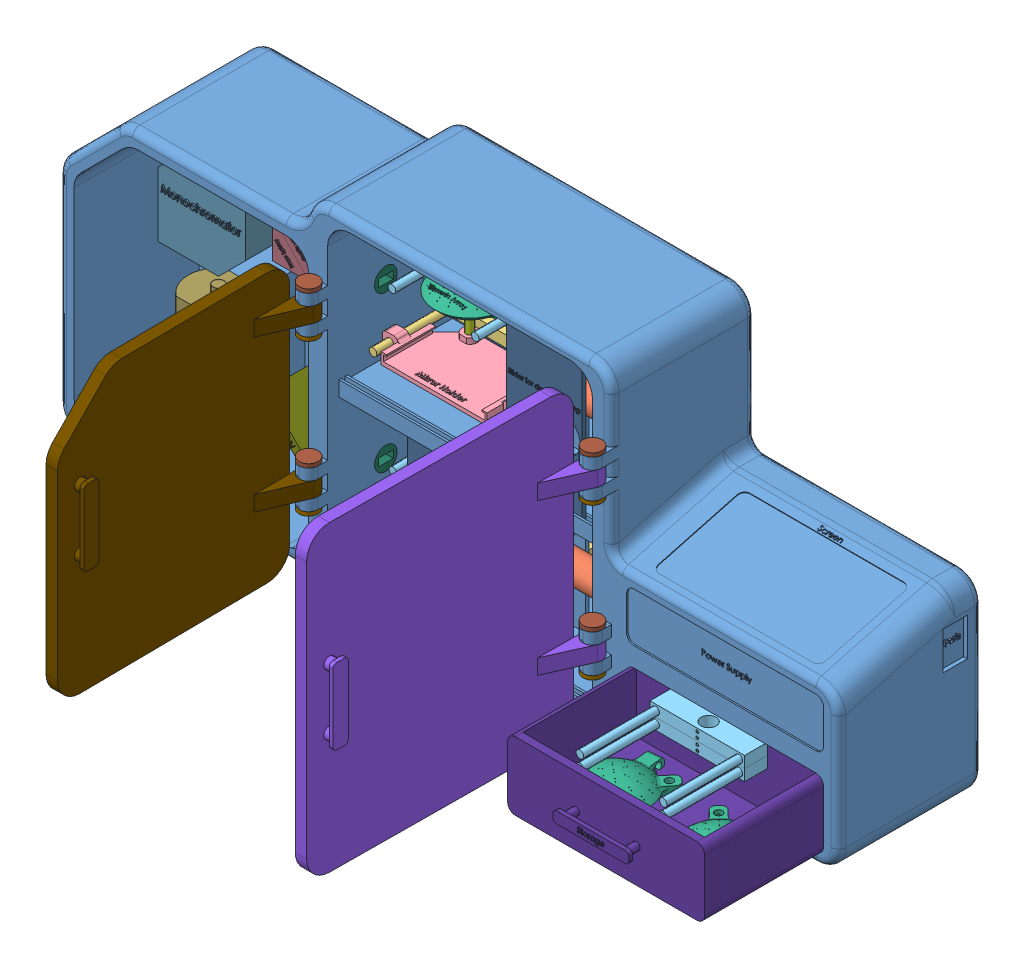
SolidWorks assembly Final Assembly of Double Beam Ultrasonic Levitator Based UV Vis Spectrophotometer, configuration Default. Lengths in mm.
Overall size (1030 440 565.09).
39 component instances, 18 part files, 70 mates.
Components (placement in the parent):
- Space for Levis-1: Space for Levis [Default] at (179.9409 252.7953 313.705) size (1030 440 215)
- Photomultiplier Tube-1: Photomultiplier Tube [Default] at (336.9409 347.7953 326.705) x (0 0 1) z (-1 0 0) size (42 42 123)
- Photomultiplier Tube-2: Photomultiplier Tube [Default] at (336.9409 142.7953 326.705) x (0 0.910058 0.414481) z (-1 0 0) size (42 42 123)
- Mirror Holder in Space for Levis-1: Mirror Holder in Space for Levis [Default] at (114.9409 294.2848 258.705) size (180 15 130)
- glassholder4-1: glassholder4 [Default] at (114.9409 293.7848 348.914) size (180 28 94.02)
- Hope4 Holder in Space for Levis-1: Hope4 Holder in Space for Levis [Default] at (114.9409 379.1402 258.705) size (125 15 130)
- hope4 (Ultrasonic Levitator Array)-1: hope4 (Ultrasonic Levitator Array) [Default] at (114.9409 389.0402 325.825) x (0 -1 0) z (-0.707107 0 0.707107) size (28.18 115.39 115.39)
- Rod-1: Rod [Default] at (78.0299 279.3165 288.914) x (0.509758 0 -0.860318) z (0.860318 0 0.509758) size (10 120 10)
- Rod-2: Rod [Default] at (151.8519 279.2413 288.914) x (0.890523 0 -0.454938) z (0.454938 0 0.890523) size (10 120 10)
- hope4 (Ultrasonic Levitator Array)-2: hope4 (Ultrasonic Levitator Array) [Default] at (116.359 182.1368 324.5152) x (0 -1 0) z (-0.691709 0 0.722177) size (28.18 115.39 115.39)
- glassholder4-2: glassholder4 [Default] at (116.8565 87.2749 347.5988) x (0.999768 0 -0.021544) z (0.021544 0 0.999768) size (180 28 94.02)
- Rod-3: Rod [Default] at (78.6614 73.5 288.408) x (0.491105 0 -0.8711) z (0.8711 0 0.491105) size (10 120 10)
- Rod-4: Rod [Default] at (152.4662 73.5126 286.8175) x (0.880515 0 -0.474018) z (0.474018 0 0.880515) size (10 120 10)
- Mirror Holder in Space for Levis-2: Mirror Holder in Space for Levis [Default] at (114.9409 87.7749 258.705) x (0.999768 0 -0.021544) z (0.021544 0 0.999768) size (180 15 130)
- Hope4 Holder in Space for Levis-2: Hope4 Holder in Space for Levis [Default] at (114.9409 172.2368 258.705) x (0.999768 0 -0.021544) z (0.021544 0 0.999768) size (125 15 130)
- Door for levis-1: Door for levis [Default] at (353.4443 252.7953 603.5992) x (-0.007984 0 0.999968) z (-0.999968 0 -0.007984) size (375 400 40)
- Down nut Levis-1: Down nut Levis [Default] at (367.4409 122.7953 416.205) size (25 55 25)
- Slider Levi-1: Slider Levi [Default] at (142.4521 150.2953 380.705) size (100 195 6)
- Up nut Levis-1: Up nut Levis [Default] at (367.4409 177.7953 416.205) size (25 55 25)
- Slider Levi-2: Slider Levi [Default] at (273.1553 355.2953 380.705) size (100 195 6)
- Up nut Levis-2: Up nut Levis [Default] at (367.4409 377.7953 416.205) size (25 55 25)
- Down nut Levis-2: Down nut Levis [Default] at (367.4409 322.7953 416.205) size (25 55 25)
- Light Source-1: Light Source [Default] at (-214.0591 72.7953 328.705) x (-1 0 0) z (0 1 0) size (80 66 160)
- Beam Splitter-1: Beam Splitter [Default] at (-95.0591 342.7953 301.705) size (50 50 52)
- Beam Splitter-2: Beam Splitter [Default] at (-95.0591 342.7953 301.705) x (-1 0 0) z (0 0 1) size (50 50 52)
- Monocromator Module-1: Monocromator Module [Default] at (-271.0645 264.3953 301.705) x (1 0 0) z (0 -1 0) size (115.36 52 120)
- Lens or Slit-1: Lens or Slit [Default] at (4.9409 346.7953 326.705) x (0 -1 0) z (-1 0 0) size (40 40 31)
- Lens or Slit-2: Lens or Slit [Default] at (4.9409 141.7953 326.705) x (0 -1 0) z (-1 0 0) size (40 40 31)
- Light Mirror-2: Light Mirror [Default] at (-91.4105 142.7886 238.705) x (-1 0 0) z (0 0 1) size (63.51 63.51 122.2)
- Storage Below Screen-1: Storage Below Screen [Default] at (529.9409 97.7953 560.7683) x (-1 0 0) z (0 0 -1) size (260 90 191)
- hope4 (Ultrasonic Levitator Array)-3: hope4 (Ultrasonic Levitator Array) [Default] at (599.9409 69.8861 480.7683) x (0 -1 0) z (0.71934 0 0.694658) size (28.18 115.39 115.39)
- hope4 (Ultrasonic Levitator Array)-4: hope4 (Ultrasonic Levitator Array) [Default] at (459.9409 69.8861 480.7683) x (0 -1 0) z (-0.773241 0 -0.634113) size (28.18 115.39 115.39)
- Hope4 Holder in Space for Levis-3: Hope4 Holder in Space for Levis [Default] at (520.3311 112.7953 415.7683) size (125 15 130)
- Hope4 Holder in Space for Levis-4: Hope4 Holder in Space for Levis [Default] at (520.3311 142.7953 415.7683) x (-1 0 0) z (0 0 1) size (125 15 130)
- Door for light module-1: Door for light module [Default] at (-18.317 252.7953 583.8259) x (0.010397 0 0.999946) z (-0.999946 0 0.010397) size (335 355 40)
- Up nut Levis-3: Up nut Levis [Default] at (-7.5591 177.7953 416.205) size (25 55 25)
- Down nut Levis-3: Down nut Levis [Default] at (-7.5591 122.7953 416.205) size (25 55 25)
- Up nut Levis-4: Up nut Levis [Default] at (-7.5591 377.7953 416.205) size (25 55 25)
- Down nut Levis-4: Down nut Levis [Default] at (-7.5591 322.7953 416.205) size (25 55 25)
Mates (geometry in assembly coordinates):
- Coincident1: coincident anti-aligned: circle of Space for Levis-1; circle of Photomultiplier Tube-1
- Coincident2: coincident anti-aligned: circle of Space for Levis-1; circle of Photomultiplier Tube-2
- Parallel2: parallel anti-aligned: plane of Space for Levis-1 through (179.9409 52.7953 238.705) normal (0 0 1); plane of Mirror Holder in Space for Levis-1 through (24.9409 309.2848 243.705) normal (0 0 -1)
- Concentric2: concentric anti-aligned: cylinder of Mirror Holder in Space for Levis-1 through (34.9409 301.7848 373.705) axis (0 0 -1) radius 5; cylinder of glassholder4-1 through (34.9409 301.7848 336.414) axis (0 0 1) radius 5
- Concentric3: concentric anti-aligned: cylinder of Mirror Holder in Space for Levis-1 through (194.9409 301.7848 373.705) axis (0 0 -1) radius 5; cylinder of glassholder4-1 through (194.9409 301.7848 336.414) axis (0 0 1) radius 5
- Parallel3: parallel anti-aligned: plane of Space for Levis-1 through (179.9409 52.7953 238.705) normal (0 0 1); plane of Hope4 Holder in Space for Levis-1 through (52.4409 394.1402 243.705) normal (0 0 -1)
- Concentric5: concentric anti-aligned: cylinder of Hope4 Holder in Space for Levis-1 through (169.9409 386.6402 373.705) axis (0 0 -1) radius 5; cylinder of hope4-1 through (169.9409 386.6402 299.825) axis (0 0 1) radius 5
- Concentric6: concentric aligned: cylinder of Hope4 Holder in Space for Levis-1 through (59.9409 386.6402 373.705) axis (0 0 -1) radius 5; cylinder of hope4-1 through (59.9409 386.6402 351.825) axis (0 0 -1) radius 5
- Concentric8: concentric anti-aligned: cylinder of glassholder4-1 through (78.0299 283.7848 288.914) axis (0 1 0) radius 5; cylinder of Rod-1 through (78.0299 399.3165 288.914) axis (0 -1 0) radius 5
- Concentric9: concentric anti-aligned: cylinder of glassholder4-1 through (151.8519 283.7848 288.914) axis (0 1 0) radius 5; cylinder of Rod-2 through (151.8519 399.2413 288.914) axis (0 -1 0) radius 5
- Concentric10: concentric aligned: cylinder of Space for Levis-1 through (114.9409 407.7953 258.705) axis (0 -1 0) radius 10; cylinder of Hope4 Holder in Space for Levis-1 through (114.9409 394.1402 258.705) axis (0 -1 0) radius 10
- Concentric11: concentric aligned: cylinder of Space for Levis-1 through (114.9409 407.7953 258.705) axis (0 -1 0) radius 10; cylinder of Mirror Holder in Space for Levis-1 through (114.9409 309.2848 258.705) axis (0 -1 0) radius 10
- Lock1: lock: unknown of Rod-1; unknown of Rod-2
- Concentric12: concentric anti-aligned: cylinder of hope4-1 through (78.0299 379.0402 288.914) axis (0 1 0) radius 5; cylinder of Rod-1 through (78.0299 399.3165 288.914) axis (0 -1 0) radius 5
- Concentric13: concentric anti-aligned: cylinder of hope4-1 through (151.8519 379.0402 288.914) axis (0 1 0) radius 5; cylinder of Rod-2 through (151.8519 399.2413 288.914) axis (0 -1 0) radius 5
- Concentric14: concentric aligned: cylinder of hope4-2 through (152.4662 172.1368 286.8175) axis (0 1 0) radius 5; cylinder of glassholder4-2 through (152.4662 77.2749 286.8175) axis (0 1 0) radius 5
- Concentric15: concentric aligned: cylinder of hope4-2 through (78.6614 172.1368 288.408) axis (0 1 0) radius 5; cylinder of glassholder4-2 through (78.6614 77.2749 288.408) axis (0 1 0) radius 5
- Concentric16: concentric anti-aligned: cylinder of hope4-2 through (78.6614 172.1368 288.408) axis (0 1 0) radius 5; cylinder of Rod-3 through (78.6614 193.5 288.408) axis (0 -1 0) radius 5
- Concentric17: concentric anti-aligned: cylinder of hope4-2 through (152.4662 172.1368 286.8175) axis (0 1 0) radius 5; cylinder of Rod-4 through (152.4662 193.5126 286.8175) axis (0 -1 0) radius 5
- Lock3: lock: unknown of Rod-3; unknown of Rod-4
- Concentric18: concentric aligned: cylinder of Mirror Holder in Space for Levis-2 through (114.9409 102.7749 258.705) axis (0 -1 0) radius 10; cylinder of Hope4 Holder in Space for Levis-2 through (114.9409 187.2368 258.705) axis (0 -1 0) radius 10
- Concentric19: concentric anti-aligned: cylinder of glassholder4-2 through (36.6057 95.2749 336.8253) axis (0.021544 0 0.999768) radius 5; cylinder of Mirror Holder in Space for Levis-2 through (37.437 95.2749 375.4018) axis (-0.021544 0 -0.999768) radius 5
- Concentric20: concentric anti-aligned: cylinder of glassholder4-2 through (196.5686 95.2749 333.3782) axis (0.021544 0 0.999768) radius 5; cylinder of Mirror Holder in Space for Levis-2 through (197.3999 95.2749 371.9547) axis (-0.021544 0 -0.999768) radius 5
- Concentric21: concentric aligned: cylinder of hope4-2 through (61.932 179.7368 351.6941) axis (-0.021544 0 -0.999768) radius 5; cylinder of Hope4 Holder in Space for Levis-2 through (62.4312 179.7368 374.8632) axis (-0.021544 0 -0.999768) radius 5
- Concentric22: concentric anti-aligned: cylinder of hope4-2 through (170.7861 179.7368 297.3363) axis (0.021544 0 0.999768) radius 5; cylinder of Hope4 Holder in Space for Levis-2 through (172.4057 179.7368 372.4933) axis (-0.021544 0 -0.999768) radius 5
- Concentric23: concentric aligned: cylinder of Space for Levis-1 through (114.9409 202.7953 258.705) axis (0 -1 0) radius 10; cylinder of Hope4 Holder in Space for Levis-2 through (114.9409 187.2368 258.705) axis (0 -1 0) radius 10
- Coincident7: coincident aligned: circle of Space for Levis-1; circle of Door for levis-1
- Coincident8: coincident anti-aligned: cylinder of Up nut Levis-2 through (367.4409 377.7953 416.205) axis (0 -1 0) radius 7.5; circle of Down nut Levis-2
- Coincident9: coincident anti-aligned: circle of Down nut Levis-1; circle of Up nut Levis-1
- Coincident10: coincident anti-aligned: circle of Space for Levis-1; circle of Up nut Levis-1
- Coincident11: coincident anti-aligned: circle of Space for Levis-1; circle of Up nut Levis-2
- Coincident12: coincident aligned: line of Space for Levis-1 through (324.9409 452.7953 380.705) axis (-1 0 0); line of Slider Levi-2 through (323.1553 452.7953 380.705) axis (-1 0 0)
- Coincident13: coincident aligned: line of Space for Levis-1 through (354.9409 247.7953 380.705) axis (-1 0 0); line of Slider Levi-1 through (192.4521 247.7953 380.705) axis (-1 0 0)
- Coincident14: coincident aligned: line of Space for Levis-1 through (34.9409 52.7953 380.705) axis (1 0 0); line of Slider Levi-1 through (92.4521 52.7953 380.705) axis (1 0 0)
- Coincident15: coincident anti-aligned: line of Space for Levis-1 through (354.9409 257.7953 380.705) axis (-1 0 0); line of Slider Levi-2 through (223.1553 257.7953 380.705) axis (1 0 0)
- Coincident16: coincident anti-aligned: circle of Up nut Levis-2; circle of Down nut Levis-2
- Parallel5: parallel aligned: plane of Light Source-1 through (-214.0591 72.7953 328.705) normal (0 -1 0); plane of Space for Levis-1 through (179.9409 37.7953 313.705) normal (0 -1 0)
- Coincident23: coincident anti-aligned: plane of Beam Splitter-1 through (-120.0591 367.7953 351.705) normal (-0.707107 -0.707107 0); plane of Beam Splitter-2 through (-70.0591 317.7953 351.705) normal (0.707107 0.707107 0)
- Coincident25: coincident anti-aligned: line of Beam Splitter-1 through (-120.0591 367.7953 351.705) axis (0.707107 -0.707107 0); line of Beam Splitter-2 through (-70.0591 317.7953 351.705) axis (-0.707107 0.707107 0)
- Coincident26: coincident: point of Beam Splitter-1; unknown of Beam Splitter-2
- Coincident27: coincident anti-aligned: plane of Space for Levis-1 through (179.9409 252.7953 301.705) normal (0 0 1); plane of Beam Splitter-2 through (-95.0591 342.7953 301.705) normal (0 0 -1)
- Coincident29: coincident aligned: line of Space for Levis-1 through (-120.0591 367.7953 301.705) axis (0 -1 0); line of Beam Splitter-2 through (-120.0591 367.7953 301.705) axis (0 -1 0)
- Coincident30: coincident aligned: line of Space for Levis-1 through (-70.0591 367.7953 301.705) axis (-1 0 0); line of Beam Splitter-1 through (-70.0591 367.7953 301.705) axis (-1 0 0)
- Coincident31: coincident aligned: line of Space for Levis-1 through (-238.0591 222.7953 296.705) axis (0 -1 0); line of Light Source-1 through (-238.0591 222.7953 296.705) axis (0 -1 0)
- Coincident32: coincident aligned: line of Space for Levis-1 through (-190.0591 222.7953 296.705) axis (-1 0 0); line of Light Source-1 through (-190.0591 222.7953 296.705) axis (-1 0 0)
- Parallel7: parallel anti-aligned: plane of Space for Levis-1 through (179.9409 52.7953 238.705) normal (0 0 1); plane of Monocromator Module-1 through (-271.0645 264.3953 301.705) normal (0 0 -1)
- Parallel8: parallel aligned: plane of Space for Levis-1 through (179.9409 37.7953 313.705) normal (0 -1 0); plane of Monocromator Module-1 through (-271.0645 264.3953 351.705) normal (0 -1 0)
- Coincident33: coincident aligned: line of Space for Levis-1 through (-155.7091 384.3953 301.705) axis (-1 0 0); line of Monocromator Module-1 through (-155.7091 384.3953 301.705) axis (-1 0 0)
- Coincident34: coincident aligned: line of Space for Levis-1 through (-271.0645 349.04 301.705) axis (0 -1 0); line of Monocromator Module-1 through (-271.0645 349.04 301.705) axis (0 -1 0)
- Parallel9: parallel aligned: plane of Lens or Slit-1 through (-20.0591 341.7953 316.705) normal (0 0 1); plane of Lens or Slit-2 through (-20.0591 136.7953 316.705) normal (0 0 1)
- Parallel10: parallel aligned: plane of Space for Levis-1 through (179.9409 52.7953 238.705) normal (0 0 1); plane of Lens or Slit-2 through (-20.0591 136.7953 316.705) normal (0 0 1)
- Coincident37: coincident aligned: circle of Space for Levis-1; circle of Lens or Slit-1
- Coincident38: coincident aligned: circle of Space for Levis-1; circle of Lens or Slit-2
- Parallel11: parallel: plane of Space for Levis-1 through (179.9409 52.7953 238.705) normal (0 0 1); plane of Light Mirror-2 through (-91.4105 142.7886 238.705) normal (0 0 -1)
- Parallel12: parallel: plane of Space for Levis-1 through (179.9409 52.7953 403.705) normal (0 1 0); plane of Light Mirror-2 through (-87.9253 121.2739 358.705) normal (0 -1 0)
- Coincident51: coincident anti-aligned: circle of Storage Below Screen-1; circle of hope4-3
- Coincident52: coincident anti-aligned: circle of Storage Below Screen-1; circle of hope4-4
- Parallel14: parallel anti-aligned: plane of Space for Levis-1 through (179.9409 297.7953 233.705) normal (0 0 1); plane of Storage Below Screen-1 through (529.9409 97.7953 390.7683) normal (0 0 -1)
- Coincident57: coincident anti-aligned: circle of Hope4 Holder in Space for Levis-3; circle of Hope4 Holder in Space for Levis-4
- Coincident58: coincident anti-aligned: line of Hope4 Holder in Space for Levis-3 through (582.8311 127.7953 400.7683) axis (-1 0 0); line of Hope4 Holder in Space for Levis-4 through (457.8311 127.7953 400.7683) axis (1 0 0)
- Coincident59: coincident anti-aligned: plane of Storage Below Screen-1 through (649.9409 142.7953 400.7683) normal (0 0 1); plane of Hope4 Holder in Space for Levis-4 through (582.8311 127.7953 400.7683) normal (0 0 -1)
- Coincident60: coincident aligned: line of Storage Below Screen-1 through (409.9409 142.7953 400.7683) axis (1 0 0); line of Hope4 Holder in Space for Levis-4 through (457.8311 142.7953 400.7683) axis (1 0 0)
- Coincident61: coincident anti-aligned: circle of Space for Levis-1; circle of Door for light module-1
- Coincident62: coincident anti-aligned: circle of Up nut Levis-4; circle of Down nut Levis-4
- Coincident63: coincident anti-aligned: circle of Up nut Levis-3; circle of Down nut Levis-3
- Coincident64: coincident anti-aligned: circle of Space for Levis-1; circle of Up nut Levis-4
- Coincident65: coincident anti-aligned: circle of Space for Levis-1; circle of Up nut Levis-3
- Coincident66: coincident aligned: line of Space for Levis-1 through (409.9409 52.7953 383.705) axis (0 0 1); line of Storage Below Screen-1 through (409.9409 52.7953 390.7683) axis (0 0 1)
- Coincident67: coincident anti-aligned: line of Space for Levis-1 through (649.9409 52.7953 403.705) axis (0 0 -1); line of Storage Below Screen-1 through (649.9409 52.7953 390.7683) axis (0 0 1)
- Coincident68: coincident anti-aligned: plane of Space for Levis-1 through (179.9409 52.7953 238.705) normal (0 0 1); plane of Light Mirror-2 through (-91.4105 142.7886 238.705) normal (0 0 -1)
